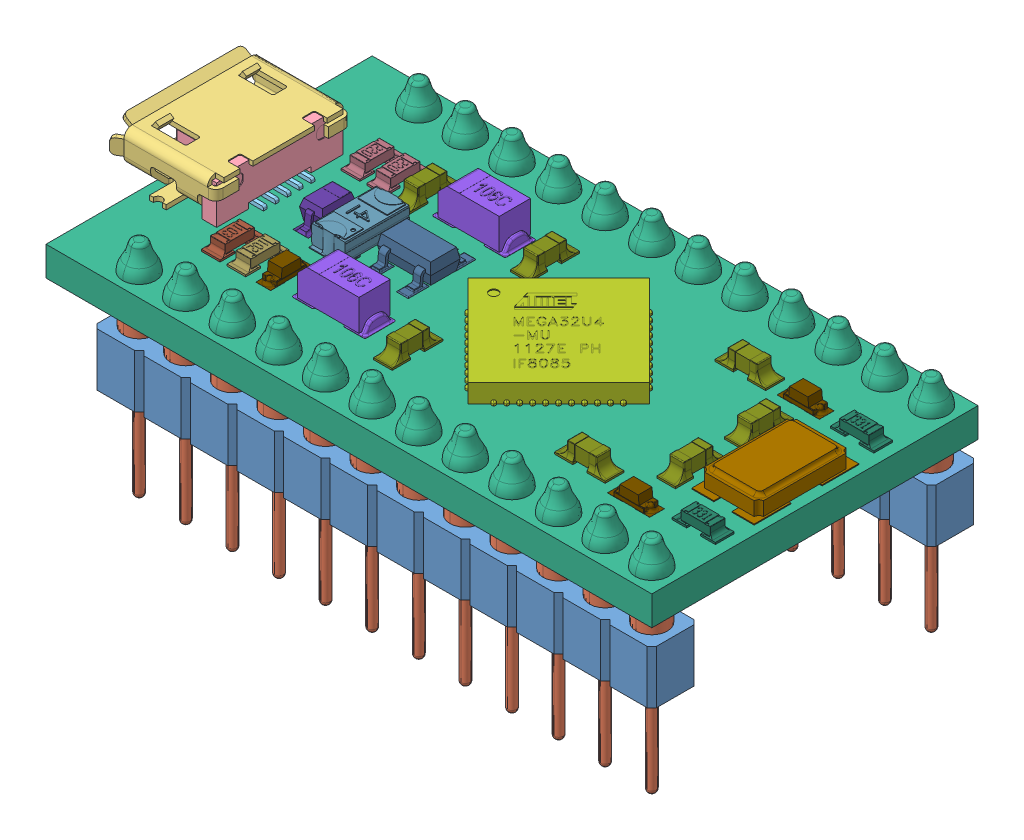
SolidWorks assembly ARDUINO PRO MICRO, configuration Default. Lengths in mm.
Overall size (34.59 13.3 17.78).
61 component instances, 18 part files, 0 mates.
Components (placement in the parent):
- ARDUINO PRO MICRO.STEP-1: ARDUINO PRO MICRO.STEP [Default] at origin size (34.59 13.3 17.78)
  - MICRO_stackable header 12.STEP-1: MICRO_stackable header 12.STEP [Default] at (0 -3.9 0) size (30.48 11.9 2.54)
    - MICRO_stackable header 12-0.STEP-1: MICRO_stackable header 12-0.STEP [Default] at origin size (30.48 2.9 2.54)
    - MICRO_stackable header pin.STEP-1: MICRO_stackable header pin.STEP [Default] at (0 3.9 0) x (0.999996 0 0.00266) z (-0.00266 0 0.999996) size (1.7 11.9 1.7)
    - MICRO_stackable header pin.STEP-2: MICRO_stackable header pin.STEP [Default] at (2.54 3.9 0) x (0.999996 0 0.00266) z (-0.00266 0 0.999996) size (1.7 11.9 1.7)
    - MICRO_stackable header pin.STEP-3: MICRO_stackable header pin.STEP [Default] at (5.08 3.9 0) x (0.999996 0 0.00266) z (-0.00266 0 0.999996) size (1.7 11.9 1.7)
    - MICRO_stackable header pin.STEP-4: MICRO_stackable header pin.STEP [Default] at (7.62 3.9 0) x (0.999996 0 0.00266) z (-0.00266 0 0.999996) size (1.7 11.9 1.7)
    - MICRO_stackable header pin.STEP-5: MICRO_stackable header pin.STEP [Default] at (10.16 3.9 0) x (0.999996 0 0.00266) z (-0.00266 0 0.999996) size (1.7 11.9 1.7)
    - MICRO_stackable header pin.STEP-6: MICRO_stackable header pin.STEP [Default] at (12.7 3.9 0) x (0.999996 0 0.00266) z (-0.00266 0 0.999996) size (1.7 11.9 1.7)
    - MICRO_stackable header pin.STEP-7: MICRO_stackable header pin.STEP [Default] at (15.24 3.9 0) x (0.999996 0 0.00266) z (-0.00266 0 0.999996) size (1.7 11.9 1.7)
    - MICRO_stackable header pin.STEP-8: MICRO_stackable header pin.STEP [Default] at (17.78 3.9 0) x (0.999996 0 0.00266) z (-0.00266 0 0.999996) size (1.7 11.9 1.7)
    - MICRO_stackable header pin.STEP-9: MICRO_stackable header pin.STEP [Default] at (20.32 3.9 0) x (0.999996 0 0.00266) z (-0.00266 0 0.999996) size (1.7 11.9 1.7)
    - MICRO_stackable header pin.STEP-10: MICRO_stackable header pin.STEP [Default] at (22.86 3.9 0) x (0.999996 0 0.00266) z (-0.00266 0 0.999996) size (1.7 11.9 1.7)
    - MICRO_stackable header pin.STEP-11: MICRO_stackable header pin.STEP [Default] at (25.4 3.9 0) x (0.999996 0 0.00266) z (-0.00266 0 0.999996) size (1.7 11.9 1.7)
    - MICRO_stackable header pin.STEP-12: MICRO_stackable header pin.STEP [Default] at (27.94 3.9 0) x (0.999996 0 0.00266) z (-0.00266 0 0.999996) size (1.7 11.9 1.7)
  - micro usb.STEP-1: micro usb.STEP [Default] at (-4.75 1.85 -7.62) x (0 0 1) z (-1 0 0) size (8 3.25 5.93)
    - micro usb shell.STEP-1: micro usb shell.STEP [Default] at origin size (8 2.95 5.63)
    - micro usb internal.STEP-1: micro usb internal.STEP [Default] at (0 -0.25 0) size (6.9 2.9 4)
    - micro usb contact.STEP-1: micro usb contact.STEP [Default] at (1.3 -0.25 -0.1) size (0.2 1.3 4.4)
    - micro usb contact.STEP-2: micro usb contact.STEP [Default] at (0.65 -0.25 -0.1) size (0.2 1.3 4.4)
    - micro usb contact.STEP-3: micro usb contact.STEP [Default] at (0 -0.25 -0.1) size (0.2 1.3 4.4)
    - micro usb contact.STEP-4: micro usb contact.STEP [Default] at (-0.65 -0.25 -0.1) size (0.2 1.3 4.4)
    - micro usb contact.STEP-5: micro usb contact.STEP [Default] at (-1.3 -0.25 -0.1) size (0.2 1.3 4.4)
  - MICRO_stackable header 12.STEP-2: MICRO_stackable header 12.STEP [Default] at (0 -3.9 -15.24) size (30.48 11.9 2.54)
    - MICRO_stackable header 12-0.STEP-1: MICRO_stackable header 12-0.STEP [Default] at origin size (30.48 2.9 2.54)
    - MICRO_stackable header pin.STEP-1: MICRO_stackable header pin.STEP [Default] at (0 3.9 0) x (0.999996 0 0.00266) z (-0.00266 0 0.999996) size (1.7 11.9 1.7)
    - MICRO_stackable header pin.STEP-2: MICRO_stackable header pin.STEP [Default] at (2.54 3.9 0) x (0.999996 0 0.00266) z (-0.00266 0 0.999996) size (1.7 11.9 1.7)
    - MICRO_stackable header pin.STEP-3: MICRO_stackable header pin.STEP [Default] at (5.08 3.9 0) x (0.999996 0 0.00266) z (-0.00266 0 0.999996) size (1.7 11.9 1.7)
    - MICRO_stackable header pin.STEP-4: MICRO_stackable header pin.STEP [Default] at (7.62 3.9 0) x (0.999996 0 0.00266) z (-0.00266 0 0.999996) size (1.7 11.9 1.7)
    - MICRO_stackable header pin.STEP-5: MICRO_stackable header pin.STEP [Default] at (10.16 3.9 0) x (0.999996 0 0.00266) z (-0.00266 0 0.999996) size (1.7 11.9 1.7)
    - MICRO_stackable header pin.STEP-6: MICRO_stackable header pin.STEP [Default] at (12.7 3.9 0) x (0.999996 0 0.00266) z (-0.00266 0 0.999996) size (1.7 11.9 1.7)
    - MICRO_stackable header pin.STEP-7: MICRO_stackable header pin.STEP [Default] at (15.24 3.9 0) x (0.999996 0 0.00266) z (-0.00266 0 0.999996) size (1.7 11.9 1.7)
    - MICRO_stackable header pin.STEP-8: MICRO_stackable header pin.STEP [Default] at (17.78 3.9 0) x (0.999996 0 0.00266) z (-0.00266 0 0.999996) size (1.7 11.9 1.7)
    - MICRO_stackable header pin.STEP-9: MICRO_stackable header pin.STEP [Default] at (20.32 3.9 0) x (0.999996 0 0.00266) z (-0.00266 0 0.999996) size (1.7 11.9 1.7)
    - MICRO_stackable header pin.STEP-10: MICRO_stackable header pin.STEP [Default] at (22.86 3.9 0) x (0.999996 0 0.00266) z (-0.00266 0 0.999996) size (1.7 11.9 1.7)
    - MICRO_stackable header pin.STEP-11: MICRO_stackable header pin.STEP [Default] at (25.4 3.9 0) x (0.999996 0 0.00266) z (-0.00266 0 0.999996) size (1.7 11.9 1.7)
    - MICRO_stackable header pin.STEP-12: MICRO_stackable header pin.STEP [Default] at (27.94 3.9 0) x (0.999996 0 0.00266) z (-0.00266 0 0.999996) size (1.7 11.9 1.7)
  - micro board.STEP-1: micro board.STEP [Default] at origin size (33.02 3.1 17.78)
  - atmega32U4.STEP-1: atmega32U4.STEP [Default] at (15.24 1.62 -7.62) x (-0.707107 0 0.707107) z (-0.707107 0 -0.707107) size (7.23 1.02 7.23)
  - MICRO_cap106C.STEP-1: MICRO_cap106C.STEP [Default] at (7.3558 1.6 -11.4427) x (0 0 -1) z (1 0 0) size (1.7 1.81 4)
  - MICRO_cap106C.STEP-2: MICRO_cap106C.STEP [Default] at (7.3558 1.6 -3.7973) x (0 0 -1) z (1 0 0) size (1.7 1.81 4)
  - micro_crystal 5x3.STEP-1: micro_crystal 5x3.STEP [Default] at (27.051 1.65 -7.62) x (0 0 -1) z (1 0 0) size (5.7 1 3.4)
  - micro_MIC5219.STEP-1: micro_MIC5219.STEP [Default] at (7.366 1.6 -7.874) x (-1 0 0) z (0 0 -1) size (2.9 1.2 3.68)
  - MICRO_603 resistor 103.STEP-1: MICRO_603 resistor 103.STEP [Default] at (1.27 1.6 -3.81) x (0 0 1) z (-1 0 0) size (2.36 0.61 1.02)
  - MICRO_603 resistor 102.STEP-1: MICRO_603 resistor 102.STEP [Default] at (2.667 1.6 -3.81) x (0 0 1) z (-1 0 0) size (2.36 0.61 1.02)
  - MICRO_603 resistor 22.STEP-1: MICRO_603 resistor 22.STEP [Default] at (1.27 1.6 -11.43) x (0 0 1) z (-1 0 0) size (2.36 0.61 1.02)
  - MICRO_603 resistor 22.STEP-2: MICRO_603 resistor 22.STEP [Default] at (2.667 1.6 -11.43) x (0 0 1) z (-1 0 0) size (2.36 0.61 1.02)
  - MICRO_PTC-1206.STEP-1: MICRO_PTC-1206.STEP [Default] at (4.445 1.6 -7.62) x (0 0 1) z (-1 0 0) size (3.85 1.17 1.82)
  - MICRO_603 resistor 331.STEP-1: MICRO_603 resistor 331.STEP [Default] at (27.432 1.6 -11.938) size (2.36 0.61 1.02)
  - MICRO_603 resistor 331.STEP-2: MICRO_603 resistor 331.STEP [Default] at (27.432 1.6 -3.302) size (2.36 0.61 1.02)
  - MICRO_603 cap on pad.STEP-1: MICRO_603 cap on pad.STEP [Default] at (24.384 1.6 -9.398) x (0 0 1) z (-1 0 0) size (2.76 0.9 1.03)
  - MICRO_603 cap on pad.STEP-2: MICRO_603 cap on pad.STEP [Default] at (21.336 1.6 -11.938) size (2.76 0.9 1.03)
  - MICRO_603 cap on pad.STEP-3: MICRO_603 cap on pad.STEP [Default] at (24.384 1.6 -5.715) x (0 0 1) z (-1 0 0) size (2.76 0.9 1.03)
  - MICRO_603 cap on pad.STEP-4: MICRO_603 cap on pad.STEP [Default] at (21.336 1.6 -3.1877) size (2.76 0.9 1.03)
  - MICRO_603 cap on pad.STEP-5: MICRO_603 cap on pad.STEP [Default] at (11.0744 1.6 -3.5839) x (0 0 -1) z (1 0 0) size (2.76 0.9 1.03)
  - MICRO_603 cap on pad.STEP-6: MICRO_603 cap on pad.STEP [Default] at (10.6528 1.6 -11.4681) x (0 0 1) z (-1 0 0) size (2.76 0.9 1.03)
  - MICRO_603 cap on pad.STEP-7: MICRO_603 cap on pad.STEP [Default] at (4.1758 1.6 -11.43) x (0 0 -1) z (1 0 0) size (2.76 0.9 1.03)
  - SOD 323.STEP-1: SOD 323.STEP [Default] at (2.6416 1.6 -7.62) x (0 0 1) z (-1 0 0) size (2.94 1.1 1.25)
  - MICRO_led.STEP-1: MICRO_led.STEP [Default] at (24.384 1.62 -2.6907) size (2.3 0.72 0.8)
  - MICRO_led.STEP-2: MICRO_led.STEP [Default] at (24.384 1.62 -11.938) size (2.3 0.72 0.8)
  - MICRO_led.STEP-3: MICRO_led.STEP [Default] at (4.1046 1.62 -3.81) x (0 0 -1) z (1 0 0) size (2.3 0.72 0.8)
